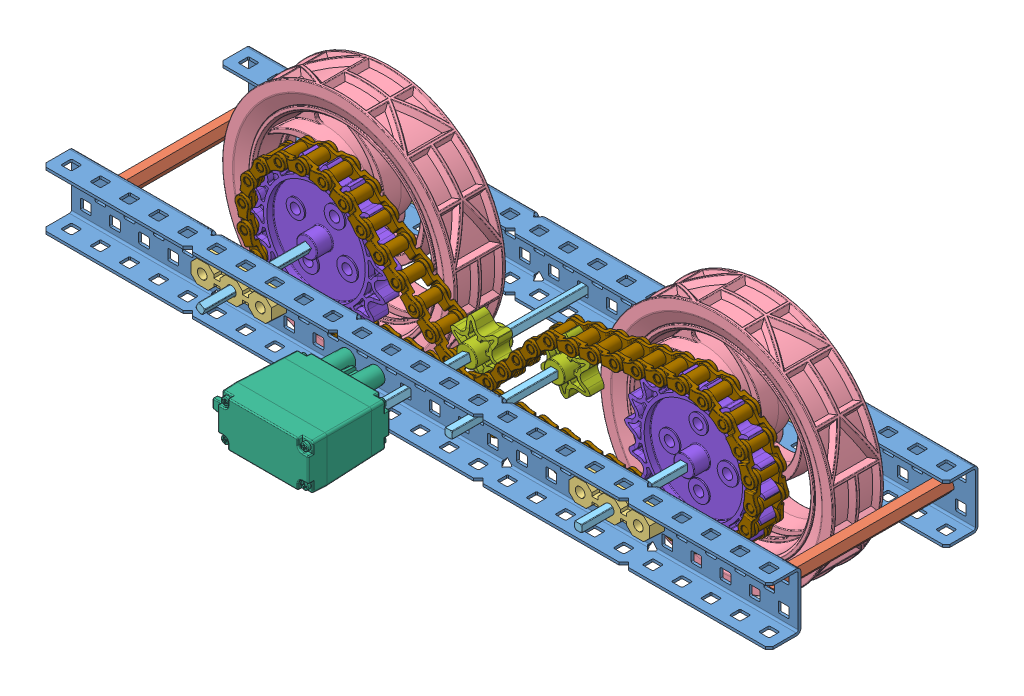
SolidWorks assembly Chassis, configuration Default. Lengths in mm.
Overall size (317.5 140.41 133.01).
74 component instances, 9 part files, 63 mates.
Components (placement in the parent):
- BaseUC-4: BaseUC [Default] at (-291.0348 15.6006 0) x (1 0 0) z (0 1 0) size (317.5 13.87 25.4)
- BEAM-3000-7: BEAM-3000 [Default] at (-304.8 12.7 -39.2684) x (1 0 0) z (0 -1 0) size (7.34 77.08 7.34)
- BEAM-3000-8: BEAM-3000 [Default] at (-12.7 12.7 -39.2684) x (-0.63784 -0.770169 0) z (-0.770169 0.63784 0) size (7.34 77.08 7.34)
- BaseUC-7: BaseUC [Default] at (-291.0348 15.6006 -77.3684) x (1 0 0) z (0 1 0) size (317.5 13.87 25.4)
- BEARING-FLAT-5: BEARING-FLAT [Default] at (-49.784 25.4 88.9762) x (0 0 -1) z (0 1 0) size (7.04 35.56 10.16)
- BEARING-FLAT-6: BEARING-FLAT [Default] at (-214.884 25.4 88.9762) x (0 0 -1) z (0 1 0) size (7.04 35.56 10.16)
- BEARING-FLAT-7: BEARING-FLAT [Default] at (-49.784 25.4 11.6078) x (0 0 -1) z (0 1 0) size (7.04 35.56 10.16)
- BEARING-FLAT-8: BEARING-FLAT [Default] at (-214.884 25.4 11.6078) x (0 0 -1) z (0 1 0) size (7.04 35.56 10.16)
- VEX-MEDIUM-WHEEL-3: VEX-MEDIUM-WHEEL [Default] at (-37.1315 -9.2154 -55.044) x (0.998133 0.061083 0) z (0 0 1) size (132.42 132.57 22.31)
- VEX-MEDIUM-WHEEL-4: VEX-MEDIUM-WHEEL [Default] at (-202.5787 -9.8231 -55.044) x (0.998965 0.045481 0) z (0 0 1) size (132.42 132.57 22.31)
- SHAFT-4000-1: SHAFT-4000 [Default] at (-241.3 12.7 -30.9) x (0.456181 0.889887 0) z (0 0 1) size (4.18 4.18 101.81)
- SHAFT-4000-2: SHAFT-4000 [Default] at (-76.2 12.7 -30.9) x (-0.999953 -0.009699 0) z (0 0 1) size (4.18 4.18 101.81)
- SHAFT-4000-3: SHAFT-4000 [Default] at (-132.8293 19.7739 -30.9) size (4.18 4.18 101.81)
- SHAFT-4000-4: SHAFT-4000 [Default] at (-171.4187 6.3323 -30.9) x (-0.963526 -0.267616 0) z (0 0 1) size (4.18 4.18 101.81)
- VEX-2WIRE-MOTOR-1: VEX-2WIRE-MOTOR [Default] at (-182.5798 6.35 43.2) size (46.4 20 51.81)
- sprocket-hs-06-tooth-1: sprocket-hs-06-tooth [Default] at (-171.4187 6.3323 -34.515) x (0.963526 0.267616 0) z (0 0 1) size (21.52 24.74 15.88)
- sprocket-hs-18-tooth-1: sprocket-hs-18-tooth [Default] at (-241.3 12.7 -34.515) x (0.889887 -0.456181 0) z (0 0 1) size (60.62 61.51 15.88)
- sprocket-hs-18-tooth-2: sprocket-hs-18-tooth [Default] at (-76.2 12.7 -34.193) x (0.009699 -0.999953 0) z (0 0 1) size (60.62 61.51 15.88)
- sprocket-hs-06-tooth-2: sprocket-hs-06-tooth [Default] at (-132.8293 19.7739 -34.193) size (21.52 24.74 15.88)
- chain-hs-link-1: chain-hs-link [Default] at (-202.7386 18.3149 -29.705) x (0.778519 -0.62762 0) z (0.62762 0.778519 0) size (15.79 14.22 6)
- chain-hs-link-3: chain-hs-link [Default] at (-210.3676 24.4652 -29.705) x (0.778519 -0.62762 0) z (0.62762 0.778519 0) size (15.79 14.22 6)
- chain-hs-link-4: chain-hs-link [Default] at (-217.9965 30.6154 -29.705) x (0.778519 -0.62762 0) z (0.62762 0.778519 0) size (15.79 14.22 6)
- chain-hs-link-5: chain-hs-link [Default] at (-225.7172 36.6501 -29.705) x (0.787882 -0.615827 0) z (0.615827 0.787882 0) size (15.79 14.22 6)
- chain-hs-link-6: chain-hs-link [Default] at (-234.7258 40.5066 -29.705) x (0.919302 -0.393552 0) z (0.393552 0.919302 0) size (15.79 14.22 6)
- chain-hs-link-7: chain-hs-link [Default] at (-244.5076 41.0926 -29.705) x (0.99821 -0.059799 0) z (0.059799 0.99821 0) size (15.79 14.22 6)
- chain-hs-link-8: chain-hs-link [Default] at (-253.9121 38.3391 -29.705) x (0.959711 0.280988 0) z (-0.280988 0.959711 0) size (15.79 14.22 6)
- chain-hs-link-9: chain-hs-link [Default] at (-261.8332 32.57 -29.705) x (0.808333 0.588725 0) z (-0.588725 0.808333 0) size (15.79 14.22 6)
- chain-hs-link-10: chain-hs-link [Default] at (-267.3392 24.4639 -29.705) x (0.561881 0.827218 0) z (-0.827218 0.561881 0) size (15.79 14.22 6)
- chain-hs-link-11: chain-hs-link [Default] at (-269.7826 14.974 -29.705) x (0.249341 0.968416 0) z (-0.968416 0.249341 0) size (15.79 14.22 6)
- chain-hs-link-12: chain-hs-link [Default] at (-268.8759 5.2168 -29.705) x (-0.092526 0.99571 0) z (-0.99571 -0.092526 0) size (15.79 14.22 6)
- chain-hs-link-13: chain-hs-link [Default] at (-264.7258 -3.6604 -29.705) x (-0.42351 0.905892 0) z (-0.905892 -0.42351 0) size (15.79 14.22 6)
- chain-hs-link-14: chain-hs-link [Default] at (-257.8204 -10.6132 -29.705) x (-0.704681 0.709524 0) z (-0.709524 -0.704681 0) size (15.79 14.22 6)
- chain-hs-link-15: chain-hs-link [Default] at (-248.9719 -14.824 -29.705) x (-0.90297 0.429704 0) z (-0.429704 -0.90297 0) size (15.79 14.22 6)
- chain-hs-link-16: chain-hs-link [Default] at (-239.2289 -15.8732 -29.705) x (-0.994251 0.107071 0) z (-0.107071 -0.994251 0) size (15.79 14.22 6)
- chain-hs-link-17: chain-hs-link [Default] at (-229.4296 -15.8732 -29.705) x (-1 0 0) z (0 -1 0) size (15.79 14.22 6)
- chain-hs-link-18: chain-hs-link [Default] at (-219.6303 -15.8732 -29.705) x (-1 0 0) z (0 -1 0) size (15.79 14.22 6)
- chain-hs-link-19: chain-hs-link [Default] at (-209.831 -15.8732 -29.705) x (-1 0 0) z (0 -1 0) size (15.79 14.22 6)
- chain-hs-link-20: chain-hs-link [Default] at (-200.0317 -15.8732 -29.705) x (-1 0 0) z (0 -1 0) size (15.79 14.22 6)
- chain-hs-link-21: chain-hs-link [Default] at (-190.2323 -15.8732 -29.705) x (-1 0 0) z (0 -1 0) size (15.79 14.22 6)
- chain-hs-link-22: chain-hs-link [Default] at (-180.433 -15.8732 -29.705) x (-1 0 0) z (0 -1 0) size (15.79 14.22 6)
- chain-hs-link-23: chain-hs-link [Default] at (-170.6337 -15.8732 -29.705) x (-1 0 0) z (0 -1 0) size (15.79 14.22 6)
- chain-hs-link-24: chain-hs-link [Default] at (-160.8344 -15.8732 -29.705) x (-1 0 0) z (0 -1 0) size (15.79 14.22 6)
- chain-hs-link-25: chain-hs-link [Default] at (-151.0351 -15.8732 -29.705) x (-1 0 0) z (0 -1 0) size (15.79 14.22 6)
- chain-hs-link-26: chain-hs-link [Default] at (-141.2357 -15.8732 -29.705) x (-1 0 0) z (0 -1 0) size (15.79 14.22 6)
- chain-hs-link-27: chain-hs-link [Default] at (-131.4364 -15.8732 -29.705) x (-1 0 0) z (0 -1 0) size (15.79 14.22 6)
- chain-hs-link-28: chain-hs-link [Default] at (-121.6371 -15.8732 -29.705) x (-1 0 0) z (0 -1 0) size (15.79 14.22 6)
- chain-hs-link-29: chain-hs-link [Default] at (-111.8378 -15.8732 -29.705) x (-1 0 0) z (0 -1 0) size (15.79 14.22 6)
- chain-hs-link-30: chain-hs-link [Default] at (-102.0385 -15.8732 -29.705) x (-1 0 0) z (0 -1 0) size (15.79 14.22 6)
- chain-hs-link-31: chain-hs-link [Default] at (-92.2391 -15.8732 -29.705) x (-1 0 0) z (0 -1 0) size (15.79 14.22 6)
- chain-hs-link-32: chain-hs-link [Default] at (-82.4398 -15.8732 -29.705) x (-1 0 0) z (0 -1 0) size (15.79 14.22 6)
- chain-hs-link-33: chain-hs-link [Default] at (-72.643 -15.651 -29.705) x (-0.999743 -0.022681 0) z (0.022681 -0.999743 0) size (15.79 14.22 6)
- chain-hs-link-34: chain-hs-link [Default] at (-63.2731 -12.7819 -29.705) x (-0.956178 -0.292786 0) z (0.292786 -0.956178 0) size (15.79 14.22 6)
- chain-hs-link-35: chain-hs-link [Default] at (-55.4237 -6.9156 -29.705) x (-0.801021 -0.598636 0) z (0.598636 -0.801021 0) size (15.79 14.22 6)
- chain-hs-link-36: chain-hs-link [Default] at (-50.0179 1.2577 -29.705) x (-0.55165 -0.834076 0) z (0.834076 -0.55165 0) size (15.79 14.22 6)
- chain-hs-link-37: chain-hs-link [Default] at (-47.6915 10.7769 -29.705) x (-0.237395 -0.971413 0) z (0.971413 -0.237395 0) size (15.79 14.22 6)
- chain-hs-link-38: chain-hs-link [Default] at (-48.7183 20.5223 -29.705) x (0.104782 -0.994495 0) z (0.994495 0.104782 0) size (15.79 14.22 6)
- chain-hs-link-39: chain-hs-link [Default] at (-52.9775 29.3476 -29.705) x (0.434634 -0.900607 0) z (0.900607 0.434634 0) size (15.79 14.22 6)
- chain-hs-link-40: chain-hs-link [Default] at (-59.968 36.2149 -29.705) x (0.713366 -0.700791 0) z (0.700791 0.713366 0) size (15.79 14.22 6)
- chain-hs-link-41: chain-hs-link [Default] at (-68.8676 40.3164 -29.705) x (0.908194 -0.41855 0) z (0.41855 0.908194 0) size (15.79 14.22 6)
- chain-hs-link-42: chain-hs-link [Default] at (-78.6297 41.1697 -29.705) x (0.996201 -0.08708 0) z (0.08708 0.996201 0) size (15.79 14.22 6)
- chain-hs-link-43: chain-hs-link [Default] at (-88.2658 39.3887 -29.705) x (0.983345 0.181751 0) z (-0.181751 0.983345 0) size (15.79 14.22 6)
- chain-hs-link-44: chain-hs-link [Default] at (-97.864 37.4131 -29.705) x (0.979467 0.201604 0) z (-0.201604 0.979467 0) size (15.79 14.22 6)
- chain-hs-link-45: chain-hs-link [Default] at (-107.4621 35.4375 -29.705) x (0.979467 0.201604 0) z (-0.201604 0.979467 0) size (15.79 14.22 6)
- chain-hs-link-46: chain-hs-link [Default] at (-117.0602 33.462 -29.705) x (0.979467 0.201604 0) z (-0.201604 0.979467 0) size (15.79 14.22 6)
- chain-hs-link-47: chain-hs-link [Default] at (-126.6583 31.4864 -29.705) x (0.979467 0.201604 0) z (-0.201604 0.979467 0) size (15.79 14.22 6)
- chain-hs-link-48: chain-hs-link [Default] at (-136.2367 29.4175 -29.705) x (0.977459 0.211124 0) z (-0.211124 0.977459 0) size (15.79 14.22 6)
- chain-hs-link-49: chain-hs-link [Default] at (-143.5877 22.9376 -29.705) x (0.750153 0.661264 0) z (-0.661264 0.750153 0) size (15.79 14.22 6)
- chain-hs-link-50: chain-hs-link [Default] at (-149.9641 15.4965 -29.705) x (0.650693 0.759341 0) z (-0.759341 0.650693 0) size (15.79 14.22 6)
- chain-hs-link-51: chain-hs-link [Default] at (-156.3404 8.0555 -29.705) x (0.650693 0.759341 0) z (-0.759341 0.650693 0) size (15.79 14.22 6)
- chain-hs-link-52: chain-hs-link [Default] at (-162.7168 0.6145 -29.705) x (0.650693 0.759341 0) z (-0.759341 0.650693 0) size (15.79 14.22 6)
- chain-hs-link-53: chain-hs-link [Default] at (-171.3638 -3.9958 -29.705) x (0.882413 0.470475 0) z (-0.470475 0.882413 0) size (15.79 14.22 6)
- chain-hs-link-54: chain-hs-link [Default] at (-180.2329 0.1714 -29.705) x (0.90507 -0.425262 0) z (0.425262 0.90507 0) size (15.79 14.22 6)
- chain-hs-link-55: chain-hs-link [Default] at (-187.8618 6.3217 -29.705) x (0.778519 -0.62762 0) z (0.62762 0.778519 0) size (15.79 14.22 6)
- chain-hs-link-56: chain-hs-link [Default] at (-195.4908 12.4719 -29.705) x (0.778519 -0.62762 0) z (0.62762 0.778519 0) size (15.79 14.22 6)
Mates (geometry in assembly coordinates):
- Coincident29: coincident anti-aligned: plane of BaseUC-4 through (-317.5 25.4 -1.1684) normal (0 0 -1); plane of BEAM-3000-7 through (-306.6331 15.875 -1.1684) normal (0 0 1)
- Coincident30: coincident anti-aligned: plane of BaseUC-4 through (-317.5 25.4 -1.1684) normal (0 0 -1); plane of BEAM-3000-8 through (-9.0855 12.0866 -1.1684) normal (0 0 1)
- Width38: width: plane of BaseUC-4 through (-15.0114 10.3886 1.3716) normal (1 0 0); plane of BaseUC-4 through (-10.3886 10.3886 1.3716) normal (-1 0 0); cylinder of BEAM-3000-8 through (-12.7 12.7 -64.6684) axis (0 0 -1) radius 2.0955
- Width39: width: plane of BaseUC-4 through (-15.0114 10.3886 1.3716) normal (0 1 0); plane of BaseUC-4 through (-15.0114 15.0114 1.3716) normal (0 -1 0); cylinder of BEAM-3000-8 through (-12.7 12.7 -64.6684) axis (0 0 -1) radius 2.0955
- Width40: width: plane of BaseUC-4 through (-302.4886 10.3886 1.3716) normal (-1 0 0); plane of BaseUC-4 through (-307.1114 10.3886 1.3716) normal (1 0 0); cylinder of BEAM-3000-7 through (-304.8 12.7 -64.6684) axis (0 0 -1) radius 2.0955
- Width41: width: plane of BaseUC-4 through (-307.1114 10.3886 1.3716) normal (0 1 0); plane of BaseUC-4 through (-307.1114 15.0114 1.3716) normal (0 -1 0); cylinder of BEAM-3000-7 through (-304.8 12.7 -64.6684) axis (0 0 -1) radius 2.0955
- Width42: width: plane of BaseUC-7 through (-302.4886 10.3886 -75.9968) normal (-1 0 0); plane of BaseUC-7 through (-307.1114 10.3886 -75.9968) normal (1 0 0); cylinder of BEAM-3000-7 through (-304.8 12.7 -64.6684) axis (0 0 -1) radius 2.0955
- Width43: width: plane of BaseUC-7 through (-307.1114 15.0114 -75.9968) normal (0 -1 0); plane of BaseUC-7 through (-307.1114 10.3886 -75.9968) normal (0 1 0); cylinder of BEAM-3000-7 through (-304.8 12.7 -64.6684) axis (0 0 -1) radius 2.0955
- Coincident33: coincident anti-aligned: plane of BEAM-3000-7 through (-306.6331 15.875 -77.3684) normal (0 0 -1); plane of BaseUC-7 through (-317.5 25.4 -77.3684) normal (0 0 1)
- Width44: width: plane of BaseUC-7 through (-15.0114 10.3886 -75.9968) normal (0 1 0); plane of BaseUC-7 through (-15.0114 15.0114 -75.9968) normal (0 -1 0); cylinder of BEAM-3000-8 through (-12.7 12.7 -64.6684) axis (0 0 -1) radius 2.0955
- Parallel11: parallel anti-aligned: line of BaseUC-4 through (-61.473 25.4 12.7) axis (1 0 0); line of BEARING-FLAT-5 through (-60.9585 17.78 0) axis (-1 0 0)
- Coincident38: coincident anti-aligned: plane of BaseUC-4 through (-317.5 25.4 0) normal (0 0 1); plane of BEARING-FLAT-5 through (-93.9837 7.6163 0) normal (0 0 -1)
- Parallel12: parallel anti-aligned: line of BaseUC-4 through (-315.8744 25.4 12.7) axis (1 0 0); line of BEARING-FLAT-6 through (-226.0585 17.78 0) axis (-1 0 0)
- Coincident39: coincident anti-aligned: plane of BaseUC-4 through (-317.5 25.4 0) normal (0 0 1); plane of BEARING-FLAT-6 through (-259.0837 7.6163 0) normal (0 0 -1)
- Parallel13: parallel anti-aligned: line of BEARING-FLAT-5 through (-60.9585 17.78 0) axis (-1 0 0); line of BaseUC-7 through (-61.473 25.4 -64.6684) axis (1 0 0)
- Parallel14: parallel anti-aligned: line of BaseUC-7 through (-61.473 25.4 -64.6684) axis (1 0 0); line of BEARING-FLAT-7 through (-60.9585 17.78 -77.3684) axis (-1 0 0)
- Coincident41: coincident anti-aligned: plane of BaseUC-7 through (-317.5 25.4 -77.3684) normal (0 0 1); plane of BEARING-FLAT-7 through (-93.9837 7.6163 -77.3684) normal (0 0 -1)
- Parallel15: parallel anti-aligned: line of BaseUC-7 through (-315.8744 1.1684 -64.6684) axis (1 0 0); line of BEARING-FLAT-8 through (-226.0585 17.78 -77.3684) axis (-1 0 0)
- Coincident42: coincident anti-aligned: plane of BaseUC-7 through (-317.5 25.4 -77.3684) normal (0 0 1); plane of BEARING-FLAT-8 through (-259.0837 7.6163 -77.3684) normal (0 0 -1)
- Width57: width: plane of BaseUC-4 through (-78.5114 10.3886 1.3716) normal (1 0 0); plane of BaseUC-4 through (-73.8886 10.3886 1.3716) normal (-1 0 0); cylinder of BEARING-FLAT-5 through (-76.2 12.7 0) axis (0 0 1) radius 2.1209
- Width58: width: plane of BaseUC-4 through (-78.5114 10.3886 1.3716) normal (0 1 0); plane of BaseUC-4 through (-78.5114 15.0114 1.3716) normal (0 -1 0); cylinder of BEARING-FLAT-5 through (-76.2 12.7 0) axis (0 0 1) radius 2.1209
- Width59: width: plane of BaseUC-7 through (-78.5114 10.3886 -75.9968) normal (0 1 0); plane of BaseUC-7 through (-78.5114 15.0114 -75.9968) normal (0 -1 0); cylinder of BEARING-FLAT-7 through (-76.2 12.7 -77.3684) axis (0 0 1) radius 2.1209
- Width60: width: plane of BaseUC-7 through (-78.5114 10.3886 -75.9968) normal (1 0 0); plane of BaseUC-7 through (-73.8886 10.3886 -75.9968) normal (-1 0 0); cylinder of BEARING-FLAT-7 through (-76.2 12.7 -77.3684) axis (0 0 1) radius 2.1209
- Width61: width: plane of BaseUC-7 through (-243.6114 10.3886 -75.9968) normal (0 1 0); plane of BaseUC-7 through (-243.6114 15.0114 -75.9968) normal (0 -1 0); cylinder of BEARING-FLAT-6 through (-241.3 12.7 0) axis (0 0 1) radius 2.1209
- Width62: width: plane of BaseUC-7 through (-243.6114 10.3886 -75.9968) normal (1 0 0); plane of BaseUC-7 through (-238.9886 10.3886 -75.9968) normal (-1 0 0); cylinder of BEARING-FLAT-8 through (-241.3 12.7 -77.3684) axis (0 0 1) radius 2.1209
- Width63: width: plane of BaseUC-7 through (-243.6114 15.0114 -75.9968) normal (0 -1 0); plane of BaseUC-7 through (-243.6114 10.3886 -75.9968) normal (0 1 0); cylinder of BEARING-FLAT-8 through (-241.3 12.7 -77.3684) axis (0 0 1) radius 2.1209
- Width64: width: plane of BaseUC-7 through (-243.6114 10.3886 -75.9968) normal (1 0 0); plane of BaseUC-7 through (-238.9886 10.3886 -75.9968) normal (-1 0 0); cylinder of BEARING-FLAT-6 through (-241.3 12.7 0) axis (0 0 1) radius 2.1209
- Width65: width: plane of VEX-MEDIUM-WHEEL-3 through (-77.711 10.992 -40.2255) normal (-0.061083 0.998133 0); plane of VEX-MEDIUM-WHEEL-3 through (-74.689 14.408 -40.2255) normal (0.061083 -0.998133 0); cylinder of BEARING-FLAT-5 through (-76.2 12.7 0) axis (0 0 1) radius 2.1209
- Width66: width: plane of VEX-MEDIUM-WHEEL-3 through (-77.908 14.211 -40.2255) normal (0.998133 0.061083 0); plane of VEX-MEDIUM-WHEEL-3 through (-74.492 11.189 -40.2255) normal (-0.998133 -0.061083 0); cylinder of BEARING-FLAT-5 through (-76.2 12.7 0) axis (0 0 1) radius 2.1209
- Width67: width: plane of VEX-MEDIUM-WHEEL-4 through (-242.8375 11.0158 -40.2255) normal (-0.045481 0.998965 0); plane of VEX-MEDIUM-WHEEL-4 through (-239.7625 14.3842 -40.2255) normal (0.045481 -0.998965 0); cylinder of BEARING-FLAT-8 through (-241.3 12.7 -77.3684) axis (0 0 1) radius 2.1209
- Width68: width: plane of VEX-MEDIUM-WHEEL-4 through (-239.6158 11.1625 -40.2255) normal (-0.998965 -0.045481 0); plane of VEX-MEDIUM-WHEEL-4 through (-242.9842 14.2375 -40.2255) normal (0.998965 0.045481 0); cylinder of BEARING-FLAT-8 through (-241.3 12.7 -77.3684) axis (0 0 1) radius 2.1209
- Width69: width: plane of SHAFT-4000-1 through (-240.6115 10.5631 19.9) normal (-0.456181 -0.889887 0); plane of SHAFT-4000-1 through (-239.1631 13.3885 19.9) normal (0.456181 0.889887 0); cylinder of BEARING-FLAT-8 through (-241.3 12.7 -77.3684) axis (0 0 1) radius 2.1209
- Width70: width: plane of SHAFT-4000-1 through (-243.4369 12.0115 19.9) normal (-0.889887 0.456181 0); plane of SHAFT-4000-1 through (-240.6115 10.5631 19.9) normal (0.889887 -0.456181 0); cylinder of BEARING-FLAT-8 through (-241.3 12.7 -77.3684) axis (0 0 1) radius 2.1209
- Width71: width: plane of SHAFT-4000-2 through (-74.5972 11.128 19.9) normal (0.009699 -0.999953 0); plane of SHAFT-4000-2 through (-74.628 14.3028 19.9) normal (-0.009699 0.999953 0); cylinder of BEARING-FLAT-7 through (-76.2 12.7 -77.3684) axis (0 0 1) radius 2.1209
- Width72: width: plane of SHAFT-4000-2 through (-77.8028 14.272 19.9) normal (-0.999953 -0.009699 0); plane of SHAFT-4000-2 through (-74.628 14.3028 19.9) normal (0.999953 0.009699 0); cylinder of BEARING-FLAT-7 through (-76.2 12.7 -77.3684) axis (0 0 1) radius 2.1209
- Coincident44: coincident anti-aligned: plane of BaseUC-7 through (-148.3614 21.3614 -75.9968) normal (0 -1 0); plane of SHAFT-4000-3 through (-134.4168 21.3614 19.9) normal (0 1 0)
- Coincident49: coincident aligned: plane of BaseUC-4 through (-317.5 25.4 0) normal (0 0 1); plane of assembly through (0 0 0) normal (0 0 1)
- Coincident50: coincident anti-aligned: plane of BaseUC-4 through (-317.5 0 0) normal (0 -1 0); plane of assembly through (0 0 0) normal (0 1 0)
- Coincident51: coincident aligned: plane of BaseUC-4 through (0 0 -1.1684) normal (1 0 0); plane of assembly through (0 0 0) normal (1 0 0)
- Coincident52: coincident anti-aligned: plane of BaseUC-4 through (-317.5 25.4 0) normal (0 0 1); plane of VEX-2WIRE-MOTOR-1 through (-182.5798 6.35 0) normal (0 0 -1)
- Width73: width: plane of BaseUC-4 through (-186.4614 8.6614 1.3716) normal (0 -1 0); plane of BaseUC-4 through (-186.4614 4.0386 1.3716) normal (0 1 0); cylinder of VEX-2WIRE-MOTOR-1 through (-184.15 6.35 -0.6) axis (0 0 -1) radius 1.3526
- Width74: width: plane of BaseUC-4 through (-181.8386 4.0386 1.3716) normal (-1 0 0); plane of BaseUC-4 through (-186.4614 4.0386 1.3716) normal (1 0 0); cone of VEX-2WIRE-MOTOR-1 through (-184.15 6.35 14.7131) axis (0 0 -1)
- Coincident53: coincident anti-aligned: plane of SHAFT-4000-4 through (-170.314 8.2868 19.9) normal (0.963526 0.267616 0); plane of VEX-2WIRE-MOTOR-1 through (-170.3276 8.3357 19.9) normal (-0.963526 -0.267616 0)
- Coincident54: coincident anti-aligned: plane of SHAFT-4000-4 through (-169.4643 5.2276 19.9) normal (0 0 1); plane of VEX-2WIRE-MOTOR-1 through (-172.5724 4.3643 19.9) normal (0 0 -1)
- Coincident55: coincident anti-aligned: plane of SHAFT-4000-4 through (-169.4643 5.2276 19.9) normal (0.267616 -0.963526 0); plane of VEX-2WIRE-MOTOR-1 through (-169.4643 5.2276 19.9) normal (-0.267616 0.963526 0)
- Distance3: distance = 10.16 mm aligned: plane of BEARING-FLAT-8 through (-247.3963 6.7369 -71.0184) normal (0 0 1); sphere of VEX-MEDIUM-WHEEL-4
- Distance4: distance = 10.16 mm aligned: plane of BEARING-FLAT-7 through (-82.2963 6.7369 -71.0184) normal (0 0 1); sphere of VEX-MEDIUM-WHEEL-3
- Coincident56: coincident anti-aligned: plane of SHAFT-4000-2 through (-77.8028 14.272 19.9) normal (-0.999953 -0.009699 0); plane of sprocket-hs-18-tooth-2 through (-77.8028 14.272 -97.693) normal (0.999953 0.009699 0)
- Coincident57: coincident anti-aligned: plane of SHAFT-4000-2 through (-74.5972 11.128 19.9) normal (0.009699 -0.999953 0); plane of sprocket-hs-18-tooth-2 through (-74.5972 11.128 -97.693) normal (-0.009699 0.999953 0)
- Coincident58: coincident aligned: circle of VEX-MEDIUM-WHEEL-3; plane of sprocket-hs-18-tooth-2 through (-76.2 12.7 -42.1305) normal (0 0 -1)
- Tangent4: tangent aligned: sphere of VEX-MEDIUM-WHEEL-4; plane of sprocket-hs-18-tooth-1 through (-241.3 12.7 -42.4525) normal (0 0 -1)
- Coincident59: coincident anti-aligned: plane of SHAFT-4000-1 through (-239.1631 13.3885 19.9) normal (0.456181 0.889887 0); plane of sprocket-hs-18-tooth-1 through (-241.9885 14.8369 -98.015) normal (-0.456181 -0.889887 0)
- Coincident60: coincident anti-aligned: plane of SHAFT-4000-1 through (-243.4369 12.0115 19.9) normal (-0.889887 0.456181 0); plane of sprocket-hs-18-tooth-1 through (-241.9885 14.8369 -98.015) normal (0.889887 -0.456181 0)
- Coincident61: coincident aligned: plane of sprocket-hs-06-tooth-1 through (-171.4187 6.3323 -26.5775) normal (0 0 1); plane of sprocket-hs-18-tooth-1 through (-241.3 12.7 -26.5775) normal (0 0 1)
- Coincident62: coincident anti-aligned: plane of SHAFT-4000-4 through (-173.3732 7.4371 19.9) normal (-0.963526 -0.267616 0); plane of sprocket-hs-06-tooth-1 through (-173.3732 7.4371 -42.4525) normal (0.963526 0.267616 0)
- Coincident63: coincident anti-aligned: plane of SHAFT-4000-4 through (-170.314 8.2868 19.9) normal (-0.267616 0.963526 0); plane of sprocket-hs-06-tooth-1 through (-173.3732 7.4371 -42.4525) normal (0.267616 -0.963526 0)
- Coincident64: coincident aligned: plane of sprocket-hs-18-tooth-2 through (-76.2 12.7 -26.2555) normal (0 0 1); plane of sprocket-hs-06-tooth-2 through (-132.8293 19.7739 -26.2555) normal (0 0 1)
- Coincident65: coincident anti-aligned: plane of SHAFT-4000-3 through (-134.4168 18.1864 19.9) normal (0 -1 0); plane of sprocket-hs-06-tooth-2 through (-134.4168 18.1864 -42.1305) normal (0 1 0)
- Coincident66: coincident anti-aligned: plane of SHAFT-4000-3 through (-134.4168 18.1864 19.9) normal (-1 0 0); plane of sprocket-hs-06-tooth-2 through (-134.4168 21.3614 -42.1305) normal (1 0 0)
- Distance5: distance = 0.2032 mm anti-aligned: plane of SHAFT-4000-3 through (-131.2418 18.1864 19.9) normal (1 0 0); plane of BaseUC-4 through (-131.0386 16.7386 1.3716) normal (-1 0 0)
- Coincident68: coincident aligned: plane of SHAFT-4000-3 through (-134.4168 21.3614 -81.7) normal (0 0 -1); plane of SHAFT-4000-4 through (-169.4643 5.2276 -81.7) normal (0 0 -1)
- Coincident69: coincident aligned: plane of SHAFT-4000-2 through (-74.5972 11.128 -81.7) normal (0 0 -1); plane of SHAFT-4000-3 through (-134.4168 21.3614 -81.7) normal (0 0 -1)
- Coincident70: coincident aligned: plane of SHAFT-4000-1 through (-243.4369 12.0115 -81.7) normal (0 0 -1); plane of SHAFT-4000-4 through (-169.4643 5.2276 -81.7) normal (0 0 -1)
